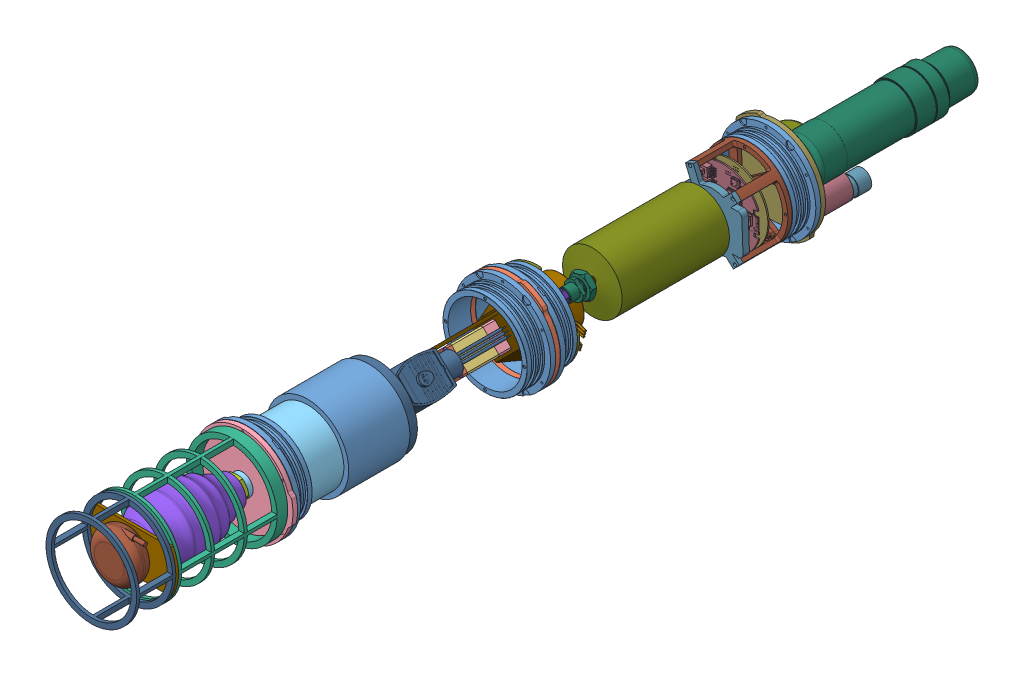
SolidWorks assembly Microfloat, configuration Default. Lengths in mm.
Overall size (181.12 175.47 1010.08).
77 component instances, 57 part files, 54 mates.
Components (placement in the parent):
- Blue Robotics - Flange - WTE4-M-FLANGE-SEAL-R3-1: Blue Robotics - Flange - WTE4-M-FLANGE-SEAL-R3 [Default] at origin size (114.3 114.3 27)
- RUR - Buoyancy Engine Assembly-1: RUR - Buoyancy Engine Assembly [Default] at (0 0 -319.175) x (0 0 1) z (-0.707107 -0.707107 0) size (229.31 105.04 98.37)
  - Takako - Pump - TFH-040-1: Takako - Pump - TFH-040 [Default] at (88.875 0 15.75) x (-1 0 0) z (0 -1 0) size (76.81 30.01 30.01)
    - 3D(TFH-040)A10-201-001-0A-IGES.IGS-1: 3D(TFH-040)A10-201-001-0A-IGES.IGS [Default] at origin size (76.81 30.01 30.01)
      - Part9.IGS-1: Part9.IGS [Default] at (3.3 0 0) x (-1 0 0) z (0 0 1) size (9.51 30.01 30.01)
      - Part10.IGS-1: Part10.IGS [Default] at (-4.2 0 0) x (1 0 0) z (0 0 -1) size (37.41 30.01 30.01)
      - Part13.IGS-1: Part13.IGS [Default] at (20.7 0 0) size (16.51 30.01 30.01)
      - Part13.1.IGS-1: Part13.1.IGS [Default] at (-3.4 0 0) x (0 1 0) z (0 0 1) size (8.05 26.51 8.05)
      - Part13.1.2.IGS-1: Part13.1.2.IGS [Default] at (40.2 0 0) size (7.01 22.01 22.01)
      - Part16.IGS-1: Part16.IGS [Default] at (47.2 0 0) size (1.01 23.01 23.01)
      - Part20.IGS-1: Part20.IGS [Default] at (-9.7 12 12) x (-1 0 0) z (0 0 1) size (53.01 5.51 5.51)
      - Part20.IGS-2: Part20.IGS [Default] at (-9.7 -12 12) x (-1 0 0) z (0 0 1) size (53.01 5.51 5.51)
      - Part20.IGS-3: Part20.IGS [Default] at (-9.7 -12 -12) x (-1 0 0) z (0 0 1) size (53.01 5.51 5.51)
      - Part20.IGS-4: Part20.IGS [Default] at (-9.7 12 -12) x (-1 0 0) z (0 0 1) size (53.01 5.51 5.51)
  - Maxon - Motor - 625857-1: Maxon - Motor - 625857 [Default] at (23.1 0 15.75) x (-1 0 0) z (0 0.5 -0.866025) size (61.3 73.93 60)
  - ASCO - Solenoid - 8262H079-1: ASCO - Solenoid - 8262H079 [Default] at (162.9914 -0.0143 22.5761) x (-1 0 0) z (0 -1 0) size (136.02 70.7 42.93)
  - RUR - Manifold-1: RUR - Manifold [Default] at (102.575 0 15.75) x (0 1 0) z (1 0 0) size (30 30 12.71)
  - Grainger - Brass Hex Nipple - 40142318-1: Grainger - Brass Hex Nipple - 40142318 [Default] at (121.4826 -0.0143 22.5761) x (-1 0 0) z (0 -0.778736 -0.627352) size (26.92 12.77 11.56)
  - McMaster - Steel Hose Fitting - 5340K11-1: McMaster - Steel Hose Fitting - 5340K11 [5340K11] at (142.1074 -0.0143 22.5761) x (0 0.556384 -0.830925) z (1 0 0) size (14.3 16.51 24.48)
  - ServoCity - Coupler - 4002-0006-0008-1: ServoCity - Coupler - 4002-0006-0008 [Default] at (35.1937 13.5518 1.5603) x (0 0.744242 -0.66791) z (0 0.66791 0.744242) size (21.24 25 20)
  - RUR - Reservoir Assembly-2: RUR - Reservoir Assembly [Default] at (-101.5 0 0) x (0 0 1) z (0 -1 0) size (73.54 44.35 104)
    - McMaster - Through Wall Fitting - 8674T54-1: McMaster - Through Wall Fitting - 8674T54 [Default] at (-28.9429 -72.9822 -1.676) x (1 0 0) z (0 -1 0) size (25.4 29.33 26.61)
    - RUR - Standoff Reservoir-1: RUR - Standoff Reservoir [Default] at (0 -101.5 0) x (0.997014 0 0.077218) z (-0.077218 0 0.997014) size (59.22 44.35 16.5) (hidden)
    - RUR - Standoff Reservoir-2: RUR - Standoff Reservoir [Default] at (0 -57.15 0) x (0.997014 0 -0.077218) z (-0.077218 0 -0.997014) size (59.22 44.35 16.5) (hidden)
    - Part1^RUR - Reservoir Assembly-1: Part1^RUR - Reservoir Assembly [Default] at origin (virtual)
  - RUR - Motor Plate V2-1: RUR - Motor Plate V2 [Default] x (0 0 -1) z (0 -1 0) size (87.12 3.17 99.5)
  - McMaster - 0.25 push fitting - 51235K107-1: McMaster - 0.25 push fitting - 51235K107 [51235K107] at (2.0922 1.676 -28.9429) x (-1 0 0) z (0 0.10178 -0.994807) size (19.14 14.66 12.7)
  - RUR - Pump Support-1: RUR - Pump Support [Default] at (3.175 0 -14.25) x (0 -1 0) z (0 0 1) size (75 129 56.15)
  - McMaster - 90 deg Push Fitting - 51235K127-1: McMaster - 90 deg Push Fitting - 51235K127 [51235K127] at (129.425 -15.6143 8.9239) x (0 1 0) z (0 0 1) size (22.01 24.69 11.7)
- Blue Robotics - Tube - WTE4-M-TUBE-12-R3-1: Blue Robotics - Tube - WTE4-M-TUBE-12-R3 [Default] at (0 0 21) x (0 0 -1) z (-0.5181 0.85532 0) size (298 111.6 111.6) (hidden)
- Blue Robotics - Flange - WTE4-M-FLANGE-SEAL-R3-2: Blue Robotics - Flange - WTE4-M-FLANGE-SEAL-R3 [Default] at (0 0 -256) x (1 0 0) z (0 0 -1) size (114.3 114.3 27)
- Blue Robotics - Flange - WTE4-M-FLANGE-SEAL-R3-3: Blue Robotics - Flange - WTE4-M-FLANGE-SEAL-R3 [Default] at (0 0 -316) size (114.3 114.3 27)
- RUR - Mid End Cap-1: RUR - Mid End Cap [Default] at (0 0 -289) x (0.5 0.866025 0) z (0 0 1) size (120.3 114.66 8.15)
- Blue Robotics - Tube - WTE4-M-TUBE-12-R3-2: Blue Robotics - Tube - WTE4-M-TUBE-12-R3 [Default] at (0 0 -295) x (0 0 -1) z (0 1 0) size (298 111.6 111.6) (hidden)
- Blue Robotics - Flange - WTE4-M-FLANGE-SEAL-R3-4: Blue Robotics - Flange - WTE4-M-FLANGE-SEAL-R3 [Default] at (0 0 -572) x (0.999281 0.037918 0) z (0 0 -1) size (114.3 114.3 27)
- McMaster - High Pressure Braided Hose - 52515K1 _ 52515K31-1: McMaster - High Pressure Braided Hose - 52515K1 _ 52515K31 [Default] at (-15.9536 -15.9738 -147.7836) x (0.70666 0.707554 0) z (-0.707554 0.70666 0) size (33.69 166.51 12.83)
- RoboSharks Bottom Cap Assembly-1: RoboSharks Bottom Cap Assembly [Default] at (0 0 27) size (120.3 114.3 199.18)
  - Bottom End Cap-1: Bottom End Cap [Default] at origin size (120.3 114.3 6)
  - RUR - Pressed Fitting Adaptor-1: RUR - Pressed Fitting Adaptor [Default] at (0 0 -13.05) x (0.700975 0.713186 0) z (0.713186 -0.700975 0) size (25.4 25.4 25.4)
  - Bellows Cage-1: Bellows Cage [Default] at (0 53.975 6) x (1 0 0) z (0 1 0) size (107.95 130.18 107.95)
  - 4810T364_British Standard Low-Pressure Stainless Steel Pipe Fitting-1: 4810T364_British Standard Low-Pressure Stainless Steel Pipe Fitting [4810T364] at (0 0 16.1424) x (0 0 -1) z (-0.004745 -0.999989 0) size (35.14 30.25 26.19)
  - Bellows-1: Bellows [Default] at (0 0 132.6472) x (-0.940852 0.338818 0) z (-0.338818 -0.940852 0) size (79.38 112.71 79.38)
  - Altimeter Attachment-1: Altimeter Attachment [Default] at (-47.625 -25.4 139.35) x (1 0 0) z (0 1 0) size (107.95 3.17 50.8)
  - Bellows Cage Extension-1: Bellows Cage Extension [Default] at (0 0 186.1292) x (1 0 0) z (0 1 0) size (107.95 46.78 107.95)
  - Altimeter-1: Altimeter [Default] at (0 0 139.35) x (1 0 0) z (0 -1 0) size (59.69 25.4 58.42)
- Sensor-Top Cap Assembly-1: Sensor-Top Cap Assembly [Default] at (-57.1134 4.1464 -711.4438) x (0.532479 -0.846444 0) z (0 0 1) size (120.3 138.3 197.96)
  - Blue Robotics End Cap-1: Blue Robotics End Cap [Default] at (33.9214 46.1354 106.4438) size (120.3 114.3 6)
  - PAR Sensor-1: PAR Sensor [Default] at (65.2064 59.4432 106.4438) x (0.464694 -0.885471 0) z (0.885471 0.464694 0) size (31.8 46.2 31.8)
  - Mini CTD-1: Mini CTD [Default] at (76.1154 32.836 17.0358) x (-0.494936 -0.868929 0) z (0.868929 -0.494936 0) size (22.35 89.41 22.35)
  - Nano with Connector-1: Nano with Connector [Default] at (25.9017 80.1424 12.1468) x (-0.308704 0.951158 0) z (-0.951158 -0.308704 0) size (55 219.9 55.03)
    - 8262-000-23_28-A.stp-1: 8262-000-23_28-A.stp [Default] at origin size (55 219.9 55.03)
      - 8262-000-28 - Nano SST final assembly with pressure PA-4LD cable connection_Substitute_2.stp-1: 8262-000-28 - Nano SST final assembly with pressure PA-4LD cable connection_Substitute_2.stp [Default] at origin size (55 219.9 55.03)
  - ECO PUCK-1: ECO PUCK [Default] at (34.0675 12.7761 52.1318) x (0.983073 -0.180853 0.029326) z (-0.183214 -0.97099 0.153661) size (63 50 63)
- BMS_Assembly-1: BMS_Assembly [Default] at (134.5929 79.8364 329.7307) x (0.720445 -0.693512 0) z (0 0 -1) size (100.72 97.29 156.69)
  - Top_Array-1: Top_Array [Default] at (-41.5993 150.8595 377.3507) x (-1 0 0) z (0 1 0) size (89.12 65 82.72)
  - Top_Bus_Half-1: Top_Bus_Half [Default] at (-41.5993 150.8595 375.3207) size (39.73 75.21 2.03)
  - Top_Case-1: Top_Case [Default] at (-41.5993 150.8595 374.3207) size (98 97.29 72.83)
  - Top_Bus_Half-2: Top_Bus_Half [Default] at (-41.5993 150.8595 377.3507) x (-1 0 0) z (0 0 -1) size (39.73 75.21 2.03)
  - Bottom_Cap-1: Bottom_Cap [Default] at (-41.5993 150.8595 302.7307) size (84.3 84.3 4.8)
  - Bottom_Bus_Full-1: Bottom_Bus_Full [Default] at (-41.5993 150.8595 304.2307) size (79.88 75.9 2.03)
  - Bottom_Array-1: Bottom_Array [Default] at (-41.5993 150.8595 306.2607) size (80.23 83.41 65)
  - Bottom Case-1: Bottom Case [Default] at (-41.5993 150.8595 306.2607) size (86.4 86.4 76.86)
  - Bottom_Bus_Half_1-1: Bottom_Bus_Half_1 [Default] at (-41.5993 150.8595 371.2607) size (45.36 69.69 2.03)
  - Bottom_Bus_Half_2-1: Bottom_Bus_Half_2 [Default] at (-41.5993 150.8595 373.2907) x (-0.809017 -0.587785 0) z (0 0 -1) size (41.78 69.69 2.03)
  - Module_Enclosure-1: Module_Enclosure [Default] at (-41.5993 150.8595 447.1507) x (-1 0 0) z (0 0 -1) size (93.94 93.19 70.5)
  - Top_Bus_Full-2: Top_Bus_Full [Default] at (-41.5993 150.8595 442.3507) size (88.77 75.21 2.03)
  - Top_Cap-2: Top_Cap [Default] at (-41.5993 150.8595 447.1507) x (1 0 0) z (0 -1 0) size (93.94 11 93.2)
- Electronics Mount Assembly Final-1: Electronics Mount Assembly Final [Default] at (-26.9756 -61.6137 -622.9532) x (0.999281 0.037918 0) z (0 0 1) size (99.82 99.82 53.34)
  - RoboSharks Electronics Mount-1: RoboSharks Electronics Mount [Default] at (29.2925 60.5466 50.9532) size (99.82 99.82 48.26)
  - SensorBoard-1: SensorBoard [Default] at (129.2925 210.5466 72.5432) x (0 -1 0) z (0 0 1) size (88.4 65 1.6)
  - ControlBoard-1: ControlBoard [Default] at (129.2925 210.5466 81.7632) x (0 -1 0) z (0 0 1) size (88.4 64.49 12.34)
  - Mount Attachment-1: Mount Attachment [Default] at (2.0115 78.6416 104.2932) x (1 0 0) z (0 0 -1) size (72.37 96.47 7.88)
  - aquabotsBMSController-1: aquabotsBMSController [Default] at (137.869 -89.4534 101.7532) x (0 1 0) z (0 0 -1) size (40 65 1.6)
- Syringe Assembly-1: Syringe Assembly [Default] at (-76.0495 -12.6781 -577.7245) x (0.705616 -0.708594 0) z (0 0 1) size (71.12 71.12 133.35)
  - Syringe-1: Syringe [Default] at (44.6781 62.8341 199.4145) size (71.12 71.12 133.35)
  - Syringe Plunger-1: Syringe Plunger [Default] at (44.6781 62.8341 139.3796) x (0.004136 -0.999991 0) z (-0.999991 -0.004136 0) size (68.58 10.16 68.58)
- Placeholder Tube 2-1: Placeholder Tube 2 [Default] at (19.2806 21.6509 -314.7661) x (0.665046 0.746803 0) z (0.746803 -0.665046 0) size (37.98 21.45 8.99)
Mates (geometry in assembly coordinates):
- Concentric3: concentric aligned: cylinder of WTE4-M-TUBE-12-R3-1 through (174.2218 -26.4485 418.6023) axis (0 0 1) radius 55.8; cylinder of WTE4-M-FLANGE-SEAL-R3-1 through (174.2218 -26.4485 141.6023) axis (0 0 1) radius 57.15
- Coincident2: coincident anti-aligned: plane of WTE4-M-TUBE-12-R3-1 through (126.1284 -11.6288 120.6023) normal (0 0 -1); plane of WTE4-M-FLANGE-SEAL-R3-1 through (179.3842 -76.3824 120.6023) normal (0 0 1)
- Concentric4: concentric anti-aligned: cylinder of WTE4-M-FLANGE-SEAL-R3-1 through (168.6712 27.2403 124.2793) axis (0 0 -1) radius 1.3; cylinder of Mid End Cap-1 through (168.6712 27.2403 114.6023) axis (0 0 1) radius 1.7
- Concentric6: concentric aligned: cylinder of Mid End Cap-1 through (196.2592 22.8227 114.6023) axis (0 0 1) radius 1.7; cylinder of WTE4-M-FLANGE-SEAL-R3-2 through (196.2592 22.8227 98.9254) axis (0 0 1) radius 1.3
- Coincident5: coincident anti-aligned: plane of WTE4-M-TUBE-12-R3-2 through (178.8177 29.1619 102.6023) normal (0 0 1); plane of WTE4-M-FLANGE-SEAL-R3-2 through (194.7179 19.3767 102.6023) normal (0 0 -1)
- Coincident6: coincident anti-aligned: plane of WTE4-M-TUBE-12-R3-2 through (178.3668 23.7055 -195.3977) normal (0 0 -1); plane of WTE4-M-FLANGE-SEAL-R3-3 through (174.2218 23.7515 -195.3977) normal (0 0 1)
- Coincident8: coincident anti-aligned: plane of WTE4-M-FLANGE-SEAL-R3-1 through (180.0989 -83.2955 114.6023) normal (0 0 -1); plane of Mid End Cap-1 through (174.2218 -26.4485 114.6023) normal (0 0 1)
- Coincident9: coincident anti-aligned: plane of Mid End Cap-1 through (174.2218 -26.4485 108.6023) normal (0 0 -1); plane of WTE4-M-FLANGE-SEAL-R3-2 through (197.5556 25.721 108.6023) normal (0 0 1)
- Concentric9: concentric anti-aligned: cylinder of Blue Robotics - Flange - WTE4-M-FLANGE-SEAL-R3-1 through (0 0 0) axis (0 0 -1) radius 44.2; cylinder of Battery Taurus-1 through (102.1027 207.4962 411.7243) axis (0 -1 0) radius 44.2
- Concentric10: concentric anti-aligned: cylinder of Blue Robotics - Flange - WTE4-M-FLANGE-SEAL-R3-1 through (0 0 0) axis (0 0 -1) radius 57.15; cylinder of Blue Robotics - Tube - WTE4-M-TUBE-12-R3-1 through (0 0 21) axis (0 0 1) radius 55.8
- Coincident13: coincident anti-aligned: plane of Blue Robotics - Flange - WTE4-M-FLANGE-SEAL-R3-1 through (0 50.2 21) normal (0 0 -1); plane of Blue Robotics - Tube - WTE4-M-TUBE-12-R3-1 through (-47.7269 -28.91 21) normal (0 0 1)
- Concentric11: concentric aligned: cylinder of Blue Robotics - Tube - WTE4-M-TUBE-12-R3-1 through (0 0 21) axis (0 0 1) radius 50.325; cylinder of Blue Robotics - Flange - WTE4-M-FLANGE-SEAL-R3-2 through (0 0 -256) axis (0 0 1) radius 50.2
- Coincident14: coincident anti-aligned: plane of Blue Robotics - Tube - WTE4-M-TUBE-12-R3-1 through (-43.044 -26.0734 -277) normal (0 0 -1); plane of Blue Robotics - Flange - WTE4-M-FLANGE-SEAL-R3-2 through (0 -50.2 -277) normal (0 0 1)
- Coincident15: coincident anti-aligned: plane of Blue Robotics - Flange - WTE4-M-FLANGE-SEAL-R3-2 through (0 -57.15 -283) normal (0 0 -1); plane of RUR - Mid End Cap-1 through (0 0 -283) normal (0 0 1)
- Concentric12: concentric aligned: cylinder of Blue Robotics - Flange - WTE4-M-FLANGE-SEAL-R3-2 through (0 0 -256) axis (0 0 1) radius 57.15; cylinder of RUR - Mid End Cap-1 through (0 0 -291.66) axis (0 0 1) radius 44.2
- Concentric13: concentric aligned: cylinder of Blue Robotics - Flange - WTE4-M-FLANGE-SEAL-R3-2 through (0 53.975 -273.323) axis (0 0 -1) radius 1.3; cylinder of RUR - Mid End Cap-1 through (0 53.975 -283) axis (0 0 -1) radius 1.6
- Coincident16: coincident anti-aligned: plane of Blue Robotics - Flange - WTE4-M-FLANGE-SEAL-R3-3 through (0 57.15 -289) normal (0 0 1); plane of RUR - Mid End Cap-1 through (0 0 -289) normal (0 0 -1)
- Concentric14: concentric aligned: cylinder of Blue Robotics - Flange - WTE4-M-FLANGE-SEAL-R3-3 through (0 0 -316) axis (0 0 -1) radius 57.15; cylinder of RUR - Mid End Cap-1 through (0 0 -283) axis (0 0 -1) radius 57.15
- Concentric15: concentric anti-aligned: cylinder of Blue Robotics - Flange - WTE4-M-FLANGE-SEAL-R3-3 through (46.7437 26.9875 -298.677) axis (0 0 1) radius 1.3; cylinder of RUR - Mid End Cap-1 through (46.7437 26.9875 -283) axis (0 0 -1) radius 1.6
- Coincident17: coincident anti-aligned: plane of Blue Robotics - Flange - WTE4-M-FLANGE-SEAL-R3-3 through (0 50.2 -295) normal (0 0 -1); plane of Blue Robotics - Tube - WTE4-M-TUBE-12-R3-2 through (-55.8 0 -295) normal (0 0 1)
- Concentric16: concentric anti-aligned: cylinder of Blue Robotics - Flange - WTE4-M-FLANGE-SEAL-R3-3 through (0 0 -316) axis (0 0 -1) radius 57.15; cylinder of Blue Robotics - Tube - WTE4-M-TUBE-12-R3-2 through (0 0 -295) axis (0 0 1) radius 55.8
- Concentric17: concentric aligned: cylinder of Blue Robotics - Tube - WTE4-M-TUBE-12-R3-2 through (0 0 -295) axis (0 0 1) radius 55.8; cylinder of Blue Robotics - Flange - WTE4-M-FLANGE-SEAL-R3-4 through (0 0 -572) axis (0 0 1) radius 57.15
- Coincident18: coincident anti-aligned: plane of Blue Robotics - Tube - WTE4-M-TUBE-12-R3-2 through (-50.325 0 -593) normal (0 0 -1); plane of Blue Robotics - Flange - WTE4-M-FLANGE-SEAL-R3-4 through (1.9035 -50.1639 -593) normal (0 0 1)
- Concentric20: concentric aligned: cylinder of Buoyancy Engine-1/Reservoir-1 through (102.1027 570.4427 411.7243) axis (0 -1 0) radius 49.53; cylinder of Battery Taurus-1 through (102.1027 207.4962 411.7243) axis (0 -1 0) radius 44.2
- Distance1: distance = 30 mm anti-aligned: plane of RUR - Buoyancy Engine Assembly-1/ASCO - Solenoid - 8262H079-1 through (-21.9376 -13.4952 -140.6336) normal (0 0 1); plane of Battery Taurus-1 through (102.1027 207.4962 411.7243) normal (0 1 0)
- Concentric22: concentric aligned: cylinder of RUR - Buoyancy Engine Assembly-1/RUR - Standoff Motor-1 through (0 46.99 -359.4247) axis (0 0 -1) radius 1.1727; cylinder of Blue Robotics - Flange - WTE4-M-FLANGE-SEAL-R3-3 through (0 46.99 -312) axis (0 0 -1) radius 1.3
- Concentric23: concentric aligned: cylinder of RUR - Buoyancy Engine Assembly-1/RUR - Standoff Motor-2 through (0 -46.99 -359.4247) axis (0 0 -1) radius 1.1727; cylinder of Blue Robotics - Flange - WTE4-M-FLANGE-SEAL-R3-3 through (0 -46.99 -312) axis (0 0 -1) radius 1.3
- Angle1: planar angle = 0.785398 rad aligned: plane of RUR - Buoyancy Engine Assembly-1/ASCO - Solenoid - 8262H079-1 through (-15.9536 -15.9738 -156.1836) normal (0.707107 -0.707107 0)
- Concentric24: concentric aligned: cylinder of RUR - Buoyancy Engine Assembly-1/ASCO - Solenoid - 8262H079-1 through (-15.9536 -15.9738 -147.6336) axis (0 0 1) radius 4.3688; cylinder of McMaster - High Pressure Braided Hose - 52515K1 & 52515K31-1 through (-15.9536 -15.9738 -147.7836) axis (0 0 1) radius 5.2022
- Coincident21: coincident anti-aligned: plane of RUR - Buoyancy Engine Assembly-1/ASCO - Solenoid - 8262H079-1 through (-21.9376 -13.4952 -140.6336) normal (0 0 1); plane of McMaster - High Pressure Braided Hose - 52515K1 & 52515K31-1 through (-15.9536 -15.9738 -140.6336) normal (0 0 -1)
- Coincident27: coordinate: point of Blue Robotics - Flange - WTE4-M-FLANGE-SEAL-R3-1
- Concentric30: concentric aligned: circle of RUR - Buoyancy Engine Assembly-1/RUR - Motor Plate V2-1; cylinder of Blue Robotics - Flange - WTE4-M-FLANGE-SEAL-R3-3 through (0 46.99 -312) axis (0 0 -1) radius 1.3
- Concentric35: concentric aligned: cylinder of RUR - Buoyancy Engine Assembly-1/RUR - Motor Plate V2-1 through (-46.99 0 -319.175) axis (0 0 -1) radius 1.7; cylinder of Blue Robotics - Flange - WTE4-M-FLANGE-SEAL-R3-3 through (-46.99 0 -312) axis (0 0 -1) radius 1.3
- Coincident28: coincident anti-aligned: plane of RUR - Buoyancy Engine Assembly-1/RUR - Motor Plate V2-1 through (0 0 -316) normal (0 0 1); plane of Blue Robotics - Flange - WTE4-M-FLANGE-SEAL-R3-3 through (0 44.2 -316) normal (0 0 -1)
- Concentric37: concentric anti-aligned: cylinder of RUR - Standoff Reservoir-1 through (44.8254 -10.329 -323.874) axis (0 0 -1) radius 1.7; cylinder of RUR - Buoyancy Engine Assembly-1/RUR - Motor Plate V2-1 through (44.8254 -10.329 -316) axis (0 0 1) radius 1.25
- Concentric39: concentric anti-aligned: cylinder of RUR - Buoyancy Engine Assembly-1/RUR - Motor Plate V2-1 through (6.8368 -45.4891 -316) axis (0 0 1) radius 1.25; circle of RUR - Standoff Reservoir-1
- Coincident30: coincident anti-aligned: plane of RUR - Buoyancy Engine Assembly-1/RUR - Motor Plate V2-1 through (0 0 -319.175) normal (0 0 -1); plane of RUR - Standoff Reservoir-1 through (22.4127 -5.1645 -319.175) normal (0 0 1)
- Coincident36: coincident anti-aligned: plane of Blue Robotics - Flange - WTE4-M-FLANGE-SEAL-R3-1 through (0 57.15 27) normal (0 0 1); plane of RoboSharks Bottom Cap Assembly-1/RUR - Bottom End Cap-1 through (0 0 27) normal (0 0 -1)
- Concentric45: concentric anti-aligned: cylinder of Blue Robotics - Flange - WTE4-M-FLANGE-SEAL-R3-1 through (-46.7437 26.9875 17.323) axis (0 0 1) radius 1.3; cylinder of RoboSharks Bottom Cap Assembly-1/RUR - Bottom End Cap-1 through (-46.7437 26.9875 33) axis (0 0 -1) radius 1.6
- Concentric46: concentric aligned: cylinder of Blue Robotics - Flange - WTE4-M-FLANGE-SEAL-R3-1 through (0 0 0) axis (0 0 -1) radius 57.15; cylinder of RoboSharks Bottom Cap Assembly-1/RUR - Bottom End Cap-1 through (0 0 33) axis (0 0 -1) radius 57.15
- Coincident37: coincident anti-aligned: plane of Blue Robotics - Flange - WTE4-M-FLANGE-SEAL-R3-4 through (2.167 -57.1089 -599) normal (0 0 -1); plane of Sensor-Top Cap Assembly-1/WTE4-M-END-CAP-R1-1 through (0 0 -599) normal (0 0 1)
- Concentric47: concentric anti-aligned: circle of Blue Robotics - Flange - WTE4-M-FLANGE-SEAL-R3-4; circle of Sensor-Top Cap Assembly-1/WTE4-M-END-CAP-R1-1
- Concentric48: concentric anti-aligned: circle of Blue Robotics - Flange - WTE4-M-FLANGE-SEAL-R3-4; circle of Sensor-Top Cap Assembly-1/WTE4-M-END-CAP-R1-1
- Concentric49: concentric anti-aligned: cylinder of Blue Robotics - Flange - WTE4-M-FLANGE-SEAL-R3-1 through (0 0 0) axis (0 0 -1) radius 44.2; cylinder of Assembly-1/Bottom_Case-1 through (0 0 -44.83) axis (0 0 1) radius 43.2
- Coincident42: coincident anti-aligned: plane of RoboSharks Bottom Cap Assembly-1/RUR - Bottom End Cap-1 through (0 0 27) normal (0 0 -1); plane of BMS_Assembly-1/Bottom_Cap-1 through (0 0 27) normal (0 0 1)
- Concentric53: concentric anti-aligned: cylinder of Blue Robotics - Flange - WTE4-M-FLANGE-SEAL-R3-1 through (0 0 0) axis (0 0 -1) radius 44.2; circle of BMS_Assembly-1/Bottom Case-1
- Concentric54: concentric anti-aligned: circle of Blue Robotics - Flange - WTE4-M-FLANGE-SEAL-R3-4; cylinder of Electronics Mount Assembly Final-1/RoboSharks Electronics Mount-1 through (1.7818 -46.9562 -566.92) axis (0 0 -1) radius 1.3834
- Concentric55: concentric anti-aligned: cylinder of Blue Robotics - Flange - WTE4-M-FLANGE-SEAL-R3-4 through (0 0 -572) axis (0 0 1) radius 50.2; cylinder of Electronics Mount Assembly Final-1/RoboSharks Electronics Mount-1 through (0 0 -566.92) axis (0 0 -1) radius 49.911
- Coincident44: coincident anti-aligned: plane of Blue Robotics - Flange - WTE4-M-FLANGE-SEAL-R3-4 through (1.676 -44.1682 -572) normal (0 0 1); plane of Electronics Mount Assembly Final-1/RoboSharks Electronics Mount-1 through (0 0 -572) normal (0 0 -1)
- Concentric56: concentric aligned: circle of Blue Robotics - Flange - WTE4-M-FLANGE-SEAL-R3-3; cylinder of Syringe Assembly-1/Syringe-1 through (0 0 -378.31) axis (0 0 1) radius 35.56
- Distance2: distance = 7 mm anti-aligned: plane of Electronics Mount Assembly Final-1/Mount Attachment-1 through (-27.9475 17.0475 -518.66) normal (0 0 1); plane of Syringe Assembly-1/Syringe-1 through (24.1956 -24.2977 -511.66) normal (0 0 -1)
- Concentric57: concentric aligned: circle of RUR - Buoyancy Engine Assembly-1/RUR - Reservoir Assembly-2/McMaster - Through Wall Fitting - 8674T54-1; circle of Placeholder Tube 2-1
- Coincident45: coincident anti-aligned: plane of RUR - Buoyancy Engine Assembly-1/RUR - Reservoir Assembly-2/McMaster - Through Wall Fitting - 8674T54-1 through (29.6501 11.2814 -356.6463) normal (0 0 -1); circle of Placeholder Tube 2-1
- Concentric58: concentric aligned: circle of Syringe Assembly-1/Syringe-1; circle of Placeholder Tube 2-1
